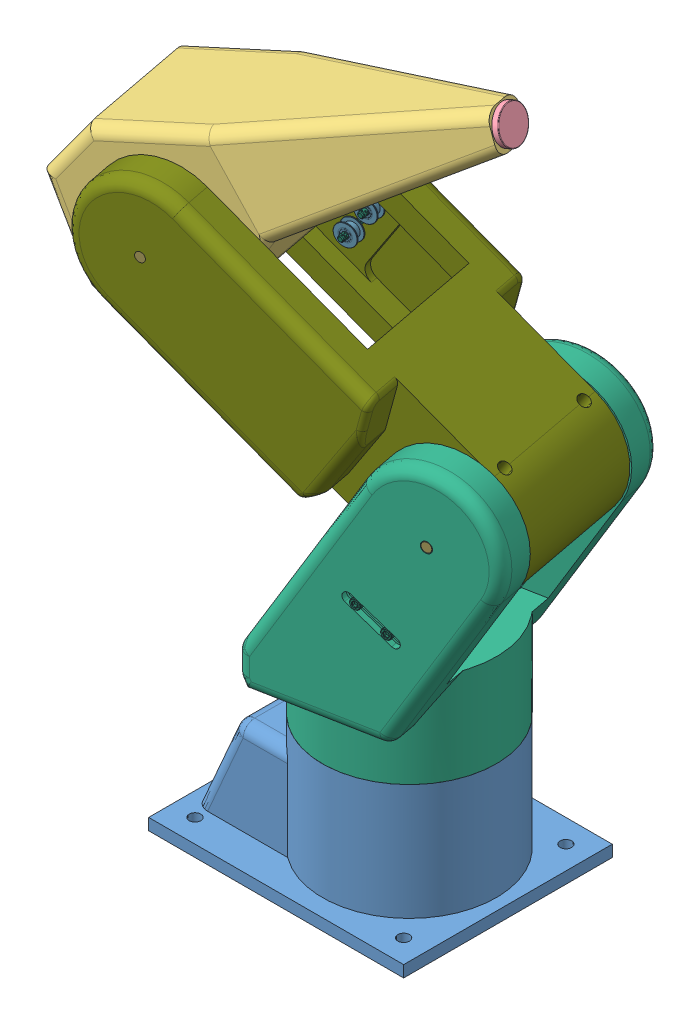
SolidWorks assembly real_of_real, configuration Default. Lengths in mm.
Overall size (412.7 619.77 234.81).
110 component instances, 22 part files, 6 mates.
Components (placement in the parent):
- Base-1: Base [Default] at (-8.9868 -21.2499 -0.8031) size (220 117.66 180)
  - base-1: base [Default] at (112.9656 83.0823 174.1461) size (220 110 180)
  - JGB37-520-12v-319RPM-1: JGB37-520-12v-319RPM [По умолчанию] at (105.1041 170.0823 173.3673) x (-0.995129 0 -0.098585) z (0 -1 0) size (36.76 36.76 71.49)
  - M3x5-2: M3x5 [Default] at (92.5422 176.0823 166.3961) x (0 -1 0) z (0 0 1) size (8 5.5 5.5)
  - M3x5-3: M3x5 [Default] at (105.9656 176.0823 158.6461) x (0 -1 0) z (0.188455 0 0.982082) size (8 5.5 5.5)
  - M3x5-6: M3x5 [Default] at (119.389 176.0823 166.3961) x (0 -1 0) z (0.395734 0 0.918365) size (8 5.5 5.5)
  - M3x5-8: M3x5 [Default] at (119.389 176.0823 181.8961) x (0 -1 0) z (0.6 0 0.8) size (8 5.5 5.5)
  - M3x5-10: M3x5 [Default] at (105.9656 176.0823 189.6461) x (0 -1 0) z (0.773678 0 0.63358) size (8 5.5 5.5)
  - M3x5-13: M3x5 [Default] at (92.5422 176.0823 181.8961) x (0 -1 0) z (0.188455 0 0.982082) size (8 5.5 5.5)
  - bearing_6809RS-1: bearing_6809RS [Default] at (144.263 164.3696 126.929) x (0 1 0) z (0 0 1) size (7 58 58)
    - ring-1: ring [Default] at (15.2127 31.2974 47.2171) size (7 58 58)
    - ball-1: ball [Default] at (15.2127 24.0864 71.9368) x (0.658873 0.218408 0.719851) z (0.355968 0.752486 -0.554123) size (4 4 4)
    - ball-2: ball [Default] at (15.2127 19.9034 70.3091) x (0.658873 0.090089 0.746841) z (0.355968 0.837276 -0.415037) size (4 4 4)
    - ball-3: ball [Default] at (15.2127 16.0666 67.9797) x (0.658873 -0.040967 0.751138) z (0.355968 0.896626 -0.26334) size (4 4 4)
    - ball-4: ball [Default] at (15.2127 12.6926 65.0195) x (0.658873 -0.170779 0.732613) z (0.355968 0.928733 -0.103642) size (4 4 4)
    - ball-5: ball [Default] at (15.2127 9.8839 61.5183) x (0.658873 -0.295401 0.691827) z (0.355968 0.932621 0.059206) size (4 4 4)
    - ball-6: ball [Default] at (15.2127 7.7259 57.5827) x (0.658873 -0.411048 0.630021) z (0.355968 0.908171 0.220254) size (4 4 4)
    - ball-7: ball [Default] at (15.2127 6.284 53.332) x (0.658873 -0.514205 0.549072) z (0.355968 0.856128 0.37461) size (4 4 4)
    - ball-8: ball [Default] at (15.2127 5.6022 48.8956) x (0.658873 -0.601739 0.45144) z (0.355968 0.778071 0.517584) size (4 4 4)
    - ball-9: ball [Default] at (15.2127 5.7011 44.4082) x (0.658873 -0.670988 0.34009) z (0.355968 0.676372 0.644831) size (4 4 4)
    - ball-10: ball [Default] at (15.2127 6.5777 40.0061) x (0.658873 -0.719851 0.218408) z (0.355968 0.554123 0.752486) size (4 4 4)
    - ball-11: ball [Default] at (15.2127 8.2054 35.8231) x (0.658873 -0.746841 0.090089) z (0.355968 0.415037 0.837276) size (4 4 4)
    - ball-12: ball [Default] at (15.2127 10.5348 31.9863) x (0.658873 -0.751138 -0.040967) z (0.355968 0.26334 0.896626) size (4 4 4)
    - ball-13: ball [Default] at (15.2127 13.495 28.6123) x (0.658873 -0.732613 -0.170779) z (0.355968 0.103642 0.928733) size (4 4 4)
    - ball-14: ball [Default] at (15.2127 16.9962 25.8036) x (0.658873 -0.691827 -0.295401) z (0.355968 -0.059206 0.932621) size (4 4 4)
    - ball-15: ball [Default] at (15.2127 20.9319 23.6456) x (0.658873 -0.630021 -0.411048) z (0.355968 -0.220254 0.908171) size (4 4 4)
    - ball-16: ball [Default] at (15.2127 25.1825 22.2037) x (0.658873 -0.549072 -0.514205) z (0.355968 -0.37461 0.856128) size (4 4 4)
    - ball-17: ball [Default] at (15.2127 29.6189 21.5219) x (0.658873 -0.45144 -0.601739) z (0.355968 -0.517584 0.778071) size (4 4 4)
    - ball-18: ball [Default] at (15.2127 34.1064 21.6208) x (0.658873 -0.34009 -0.670988) z (0.355968 -0.644831 0.676372) size (4 4 4)
    - ball-19: ball [Default] at (15.2127 38.5084 22.4974) x (0.658873 -0.218408 -0.719851) z (0.355968 -0.752486 0.554123) size (4 4 4)
    - ball-20: ball [Default] at (15.2127 42.6914 24.1251) x (0.658873 -0.090089 -0.746841) z (0.355968 -0.837276 0.415037) size (4 4 4)
    - ball-21: ball [Default] at (15.2127 46.5282 26.4545) x (0.658873 0.040967 -0.751138) z (0.355968 -0.896626 0.26334) size (4 4 4)
    - ball-22: ball [Default] at (15.2127 49.9022 29.4147) x (0.658873 0.170779 -0.732613) z (0.355968 -0.928733 0.103642) size (4 4 4)
    - ball-23: ball [Default] at (15.2127 52.7109 32.9159) x (0.658873 0.295401 -0.691827) z (0.355968 -0.932621 -0.059206) size (4 4 4)
    - ball-24: ball [Default] at (15.2127 54.869 36.8516) x (0.658873 0.411048 -0.630021) z (0.355968 -0.908171 -0.220254) size (4 4 4)
    - ball-25: ball [Default] at (15.2127 56.3108 41.1022) x (0.658873 0.514205 -0.549072) z (0.355968 -0.856128 -0.37461) size (4 4 4)
    - ball-26: ball [Default] at (15.2127 56.9927 45.5386) x (0.658873 0.601739 -0.45144) z (0.355968 -0.778071 -0.517584) size (4 4 4)
    - ball-27: ball [Default] at (15.2127 56.8937 50.0261) x (0.658873 0.670988 -0.34009) z (0.355968 -0.676372 -0.644831) size (4 4 4)
    - ball-28: ball [Default] at (15.2127 56.0171 54.4281) x (0.658873 0.719851 -0.218408) z (0.355968 -0.554123 -0.752486) size (4 4 4)
    - ball-29: ball [Default] at (15.2127 54.3894 58.6111) x (0.658873 0.746841 -0.090089) z (0.355968 -0.415037 -0.837276) size (4 4 4)
    - ball-30: ball [Default] at (15.2127 52.06 62.4479) x (0.658873 0.751138 0.040967) z (0.355968 -0.26334 -0.896626) size (4 4 4)
    - ball-31: ball [Default] at (15.2127 49.0998 65.8219) x (0.658873 0.732613 0.170779) z (0.355968 -0.103642 -0.928733) size (4 4 4)
    - ball-32: ball [Default] at (15.2127 45.5986 68.6306) x (0.658873 0.691827 0.295401) z (0.355968 0.059206 -0.932621) size (4 4 4)
    - ball-33: ball [Default] at (15.2127 41.663 70.7887) x (0.658873 0.630021 0.411048) z (0.355968 0.220254 -0.908171) size (4 4 4)
    - ball-34: ball [Default] at (15.2127 37.4123 72.2305) x (0.658873 0.549072 0.514205) z (0.355968 0.37461 -0.856128) size (4 4 4)
    - ball-35: ball [Default] at (15.2127 32.9759 72.9123) x (0.658873 0.45144 0.601739) z (0.355968 0.517584 -0.778071) size (4 4 4)
    - ball-36: ball [Default] at (15.2127 28.4885 72.8134) x (0.658873 0.34009 0.670988) z (0.355968 0.644831 -0.676372) size (4 4 4)
    - ball-37: ball [Default] at (15.2127 24.0864 71.9368) x (0.658873 0.218408 0.719851) z (0.355968 0.752486 -0.554123) size (4 4 4)
    - ball-38: ball [Default] at (15.2127 19.9034 70.3091) x (0.658873 0.090089 0.746841) z (0.355968 0.837276 -0.415037) size (4 4 4)
    - ball-39: ball [Default] at (15.2127 16.0666 67.9797) x (0.658873 -0.040967 0.751138) z (0.355968 0.896626 -0.26334) size (4 4 4)
    - ball-40: ball [Default] at (15.2127 12.6926 65.0195) x (0.658873 -0.170779 0.732613) z (0.355968 0.928733 -0.103642) size (4 4 4)
- Part1-1: Part1 [Default] at (87.1555 51.7331 -12.3821) x (0.982402 0 -0.186779) z (0.186779 0 0.982402) size (201.64 265.15 170)
  - Part1-1: Part1 [Default] at (-18.1622 110.0992 185.599) size (201.64 265.15 170)
  - Flange_6mm-1: Flange_6mm [Default] at (-18.1622 106.0992 185.599) x (-0.707107 0 0.707107) z (-0.707107 0 -0.707107) size (22 12 22)
  - M3x5-1: M3x5 [Default] at (-23.8191 103.0992 191.2558) x (0 1 0) z (0 0 1) size (8 5.5 5.5)
  - M3x5-2: M3x5 [Default] at (-23.8191 103.0992 179.9421) x (0 1 0) z (-1 0 0) size (8 5.5 5.5)
  - M3x5-3: M3x5 [Default] at (-12.5054 103.0992 179.9421) x (0 1 0) z (0 0 -1) size (8 5.5 5.5)
  - M3x5-4: M3x5 [Default] at (-12.5054 103.0992 191.2558) x (0 1 0) z (1 0 0) size (8 5.5 5.5)
  - Ball Bearing 8mm I.D, 22mm O.D-1: Ball Bearing 8mm I.D, 22mm O.D [Default] at (52.1903 311.9534 264.099) size (22 22 7)
  - Ball Bearing 8mm I.D, 22mm O.D-2: Ball Bearing 8mm I.D, 22mm O.D [Default] at (52.1903 311.9534 107.099) size (22 22 7)
  - Puly GT2 40 trục 8mm-1: Puly GT2 40 trục 8mm [Default] at (-18.1622 165.0992 253.299) x (1 0 0) z (0 1 0) size (24.8 17.3 24.8)
  - Nema17 motor support-2: Nema17 motor support [Default] at (-43.1622 135.0992 235.599) x (0 0 -1) z (1 0 0) size (53 51 50)
  - M3x5-5: M3x5 [Default] at (-28.7688 175.7058 238.599) x (0 0 -1) z (1 0 0) size (8 5.5 5.5)
  - M3x5-7: M3x5 [Default] at (-7.5556 175.7058 238.599) x (0 0 -1) z (0.987351 0.158553 0) size (8 5.5 5.5)
  - M3x5-9: M3x5 [Default] at (-7.5556 154.4926 238.599) x (0 0 -1) z (0.959125 0.282984 0) size (8 5.5 5.5)
  - M3x5-11: M3x5 [Default] at (-28.7688 154.4926 238.599) x (0 0 -1) z (0.928571 0.371154 0) size (8 5.5 5.5)
  - Nema17-gear-3: Nema17-gear [Default] at (-18.1622 165.0992 206.299) x (-1 0 0) z (0 0 1) size (42.88 42 87.3)
  - bar_170mm-1: bar_170mm [Default] at (52.1903 311.9534 100.599) size (8 8 170)
  - Pulley 80 8mm-1: Pulley 80 8mm [Default] at (52.1903 311.9534 252.599) x (1 0 0) z (0 1 0) size (55 14 55)
  - GT2 - 20T_Tension Pulley Without Teeth+603ZZ _dzino-2: GT2 - 20T_Tension Pulley Without Teeth+603ZZ _dzino [Výchozí] at (-0.6544 248.2367 246.099) x (-0.879149 -0.476547 0) z (-0.476547 0.879149 0) size (18 8.5 18)
  - GT2 - 20T_Tension Pulley Without Teeth+603ZZ _dzino-4: GT2 - 20T_Tension Pulley Without Teeth+603ZZ _dzino [Výchozí] at (22.3448 234.9582 246.099) x (-0.999765 -0.0217 0) z (-0.0217 0.999765 0) size (18 8.5 18)
  - M5x25-1: M5x25 [Default] at (22.3448 234.9582 270.599) x (0 0 -1) z (0.56919 0.822206 0) size (30.03 8.5 8.5)
  - M5x25-2: M5x25 [Default] at (-0.6544 248.2367 270.599) x (0 0 -1) z (0.755153 0.655549 0) size (30.03 8.5 8.5)
- Part2-1: Part2 [Default] at (352.0989 549.2345 -5.9554) x (0.186779 0 0.982402) z (-0.522922 -0.846562 0.09942) size (170 359.61 110)
  - Part2-1: Part2 [Default] at (184.7996 161.3802 267.2035) size (170 359.61 110)
  - Nema17 motor support-1: Nema17 motor support [Default] at (88.827 136.3802 297.2035) x (1 0 0) z (0 1 0) size (53 51 50)
  - nema17-34-1: nema17-34 [Default] at (154.696 127.2402 289.9023) x (0 0 -1) z (0 1 0) size (48.3 64 42.3)
  - Puly GT2 20 trục 5mm-1: Puly GT2 20 trục 5mm [Конфигурация1] at (82.827 161.3802 267.2035) x (-1 0 0) z (0 0 1) size (16 16 16)
  - bar_170mm-1: bar_170mm [Default] at (44.7996 325.9891 267.2035) x (0 0 -1) z (1 0 0) size (8 8 170)
  - Ball Bearing 8mm I.D, 22mm O.D-1: Ball Bearing 8mm I.D, 22mm O.D [Default] at (51.2996 325.9891 267.2035) x (0 0 -1) z (1 0 0) size (22 22 7)
  - Ball Bearing 8mm I.D, 22mm O.D-2: Ball Bearing 8mm I.D, 22mm O.D [Default] at (208.2996 325.9891 267.2035) x (0 -0.984808 0.173648) z (-1 0 0) size (22 22 7)
  - Pulley 80 8mm-1: Pulley 80 8mm [Default] at (67.827 325.9891 267.2035) x (0 -1 0) z (0 0 1) size (55 14 55)
  - Flange_8mm-1: Flange_8mm [Default] at (180.7996 76.3802 267.2035) x (0 0 1) z (0 -1 0) size (32 13 32)
  - Flange_8mm-2: Flange_8mm [Default] at (78.7996 76.3802 267.2035) x (0 0 1) z (0 1 0) size (32 13 32)
  - M4 CUP HEAD SCREW-1: M4 CUP HEAD SCREW [Default] at (88.7996 84.8655 258.7182) x (0 1 0) z (0 0 1) size (6.85 14.06 6.85)
  - M4 CUP HEAD SCREW-4: M4 CUP HEAD SCREW [Default] at (88.7996 84.8655 275.6888) x (0 0.987351 0.158553) z (0 -0.158553 0.987351) size (6.85 14.06 6.85)
  - M4 CUP HEAD SCREW-6: M4 CUP HEAD SCREW [Default] at (88.7996 67.895 275.6888) x (0 0.959125 0.282984) z (0 -0.282984 0.959125) size (6.85 14.06 6.85)
  - M4 CUP HEAD SCREW-8: M4 CUP HEAD SCREW [Default] at (88.7996 67.895 258.7182) x (0 0.928571 0.371154) z (0 -0.371154 0.928571) size (6.85 14.06 6.85)
  - M4 CUP HEAD SCREW-10: M4 CUP HEAD SCREW [Default] at (170.7996 84.8655 275.6888) x (0 0.642788 0.766044) z (0 0.766044 -0.642788) size (6.85 14.06 6.85)
  - M4 CUP HEAD SCREW-12: M4 CUP HEAD SCREW [Default] at (170.7996 84.8655 258.7182) x (0 0.766044 0.642788) z (0 0.642788 -0.766044) size (6.85 14.06 6.85)
  - M4 CUP HEAD SCREW-14: M4 CUP HEAD SCREW [Default] at (170.7996 67.895 258.7182) x (0 0.866025 0.5) z (0 0.5 -0.866025) size (6.85 14.06 6.85)
  - M4 CUP HEAD SCREW-16: M4 CUP HEAD SCREW [Default] at (170.7996 67.895 275.6888) x (0 0.939693 0.34202) z (0 0.34202 -0.939693) size (6.85 14.06 6.85)
  - GT2 - 20T_Tension Pulley Without Teeth+603ZZ _dzino-2: GT2 - 20T_Tension Pulley Without Teeth+603ZZ _dzino [Výchozí] at (69.2996 256.1847 279.9125) x (0 -0.248896 -0.96853) z (0 0.96853 -0.248896) size (18 8.5 18)
  - GT2 - 20T_Tension Pulley Without Teeth+603ZZ _dzino-3: GT2 - 20T_Tension Pulley Without Teeth+603ZZ _dzino [Výchozí] at (69.2996 256.1847 252.0738) x (0 0.542384 -0.840131) z (0 0.840131 0.542384) size (18 8.5 18)
  - M5x25-1: M5x25 [Default] at (44.7996 256.1847 252.0738) x (1 0 0) z (0 -0.923005 0.384788) size (30.03 8.5 8.5)
  - M5x25-2: M5x25 [Default] at (44.7996 256.1847 279.9125) x (1 0 0) z (0 -0.972339 0.233576) size (30.03 8.5 8.5)
- Part3-1: Part3 [Default] at (-49.2096 309.7174 -38.9153) x (0.894808 0.412767 -0.170125) z (0.186779 0 0.982402) size (337.83 131.2 113.15)
  - Part3-1: Part3 [Default] at (49.6936 182.6029 292.1353) size (332.95 131.2 113.15)
  - Flange_8mm-1: Flange_8mm [Default] at (49.6936 182.6029 186.1353) x (1 0 0) z (0 -1 0) size (32 13 32)
  - Flange_8mm-2: Flange_8mm [Default] at (49.6936 182.6029 288.1353) x (1 0 0) z (0 1 0) size (32 13 32)
  - M4 CUP HEAD SCREW-1: M4 CUP HEAD SCREW [Default] at (58.1788 191.0882 196.1353) x (-0.349376 0.936983 0) z (-0.936983 -0.349376 0) size (6.85 14.06 6.85)
  - M4 CUP HEAD SCREW-2: M4 CUP HEAD SCREW [Default] at (41.2083 191.0882 196.1353) x (-0.493517 0.869736 0) z (-0.869736 -0.493517 0) size (6.85 14.06 6.85)
  - M4 CUP HEAD SCREW-4: M4 CUP HEAD SCREW [Default] at (41.2083 174.1176 196.1353) x (-0.600246 0.799816 0) z (-0.799816 -0.600246 0) size (6.85 14.06 6.85)
  - M4 CUP HEAD SCREW-6: M4 CUP HEAD SCREW [Default] at (58.1788 174.1176 196.1353) x (0.974481 0.224471 0) z (-0.224471 0.974481 0) size (6.85 14.06 6.85)
  - M4 CUP HEAD SCREW-8: M4 CUP HEAD SCREW [Default] at (58.1788 191.0882 278.1353) x (0.942345 0.334644 0) z (0.334644 -0.942345 0) size (6.85 14.06 6.85)
  - M4 CUP HEAD SCREW-10: M4 CUP HEAD SCREW [Default] at (58.1788 174.1176 278.1353) x (0.869918 0.493196 0) z (0.493196 -0.869918 0) size (6.85 14.06 6.85)
  - M4 CUP HEAD SCREW-12: M4 CUP HEAD SCREW [Default] at (58.1788 174.1176 278.1353) x (-0.359289 -0.933226 0) z (-0.933226 0.359289 0) size (6.85 14.06 6.85)
  - M4 CUP HEAD SCREW-14: M4 CUP HEAD SCREW [Default] at (41.2083 174.1176 278.1353) x (-0.270431 -0.962739 0) z (-0.962739 0.270431 0) size (6.85 14.06 6.85)
  - M4 CUP HEAD SCREW-16: M4 CUP HEAD SCREW [Default] at (41.2083 191.0882 278.1353) x (-0.114365 -0.993439 0) z (-0.993439 0.114365 0) size (6.85 14.06 6.85)
  - Electronic_magnet_30x22-1: Electronic_magnet_30x22 [Default] at (304.3014 216.705 237.1353) x (0.090019 0.99594 0) z (0 0 1) size (30 22 30)
Mates (geometry in assembly coordinates):
- Concentric1: concentric aligned: cylinder of Base-1/JGB37-520-12v-319RPM-1 through (103.9788 169.4923 173.343) axis (0 -1 0) radius 3; cylinder of Part1-1/Flange_6mm-1 through (103.9788 169.8323 173.343) axis (0 -1 0) radius 3
- Coincident1: coincident anti-aligned: plane of Base-1/base-1 through (103.9788 154.8323 173.343) normal (0 1 0); plane of Part1-1/Part1-1 through (103.9788 154.8323 173.343) normal (0 -1 0)
- Concentric2: concentric aligned: cylinder of Part1-1/bar_170mm-1 through (188.9694 363.6865 243.7068) axis (-0.186779 0 -0.982402) radius 4; cylinder of Part2-1/Flange_8mm-1 through (182.619 363.6865 210.3052) axis (-0.186779 0 -0.982402) radius 4
- Coincident2: coincident anti-aligned: plane of Part1-1/Part1-1 through (183.3661 363.6865 214.2348) normal (-0.186779 0 -0.982402); plane of Part2-1/Part2-1 through (183.3661 363.6865 214.2348) normal (0.186779 0 0.982402)
- Coincident3: coincident anti-aligned: plane of Part2-1/Part2-1 through (-24.2248 496.5507 253.7028) normal (-0.186779 0 -0.982402); plane of Part3-1/Part3-1 through (-24.2248 496.5507 253.7028) normal (0.186779 0 0.982402)
- Concentric3: concentric aligned: cylinder of Part2-1/bar_170mm-1 through (-18.6214 496.5507 283.1749) axis (-0.186779 0 -0.982402) radius 4; cylinder of Part3-1/Flange_8mm-2 through (-24.9719 496.5507 249.7732) axis (-0.186779 0 -0.982402) radius 4
